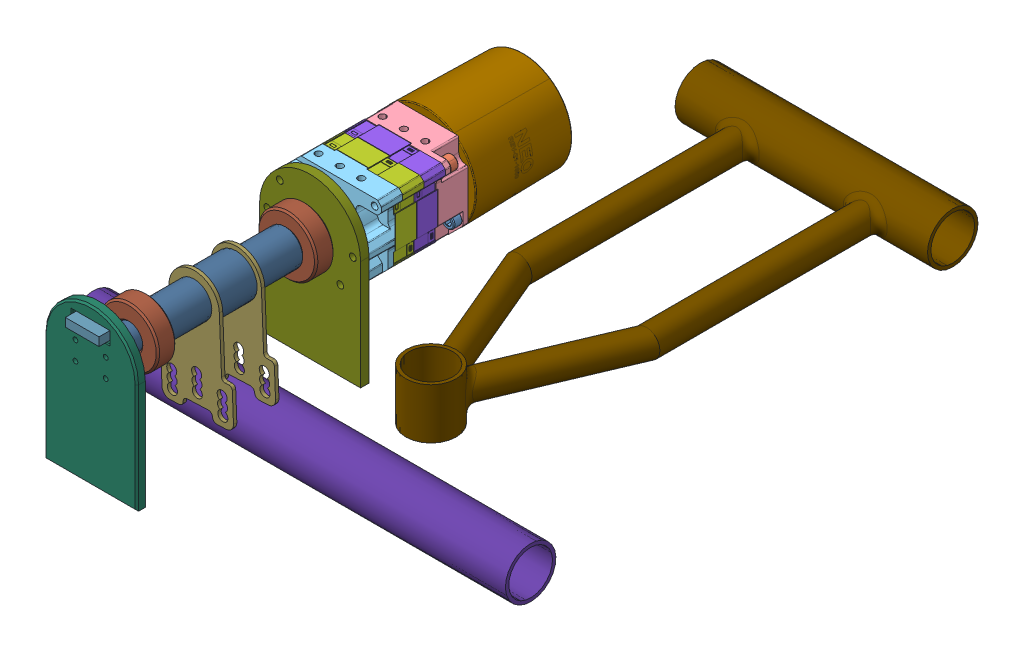
SolidWorks assembly SBW lower asm, configuration Default. Lengths in mm.
Overall size (260 177.93 457.25).
26 component instances, 18 part files, 28 mates.
Components (placement in the parent):
- MAXPlanetary 2-Stage-1: MAXPlanetary 2-Stage [Default] at origin size (89.61 89.51 122.08)
  - MAXPlanetary 2-Stage.STEP-1: MAXPlanetary 2-Stage.STEP [Default] at origin size (89.61 89.51 122.08)
    - REV-25-2109_2-Stage (No Shaft, For NEO).STEP-1: REV-25-2109_2-Stage (No Shaft, For NEO).STEP [Default] at origin size (65.15 54.03 73.34)
      - REV-25-2107_2-Stage.STEP-1: REV-25-2107_2-Stage.STEP [Default] at (0 0 6.35) x (-1 0 0) z (0 0 -1) size (65.15 54.03 73.34)
        - #10 Socket Head Cap Screws_0.500in Long.STEP-1: #10 Socket Head Cap Screws_0.500in Long.STEP [Default] at (21.1355 14.0872 12.7) x (0.923728 0.383049 0) z (0.383049 -0.923728 0) size (7.94 17.53 7.94)
        - #10 Socket Head Cap Screws_0.500in Long.STEP-2: #10 Socket Head Cap Screws_0.500in Long.STEP [Default] at (-21.1355 -14.0872 12.7) x (0.923728 0.383049 0) z (0.383049 -0.923728 0) size (7.94 17.53 7.94)
        - #10 Socket Head Cap Screws_1.500in Long.STEP-1: #10 Socket Head Cap Screws_1.500in Long.STEP [Default] at (-26.9919 21.4312 0) x (0.777574 0.628792 0) z (-0.628792 0.777574 0) size (7.94 42.93 7.94)
        - #10 Socket Head Cap Screws_1.500in Long.STEP-2: #10 Socket Head Cap Screws_1.500in Long.STEP [Default] at (26.9919 -21.4312 0) x (0.777574 0.628792 0) z (-0.628792 0.777574 0) size (7.94 42.93 7.94)
        - #10-32 Button Head Cap Screws_0.500in Long.STEP-1: #10-32 Button Head Cap Screws_0.500in Long.STEP [Default] at (0 0 -35.2425) x (0.655967 -0.754789 0) z (-0.754789 -0.655967 0) size (9.17 15.27 9.17)
      - REV-21-2106.STEP-1: REV-21-2106.STEP [Default] at origin size (61.91 50.8 19.05)
      - REV-21-2104.STEP-1: REV-21-2104.STEP [Default] at (0 0 44.45) x (0 0 1) z (-1 0 0) size (23.2 50.8 61.92)
      - REV-21-2108.STEP-1: REV-21-2108.STEP [Default] at (0 0 7.0985) x (-0.554615 -0.832107 0) z (0 0 -1) size (25.4 25.4 14.94)
    - REV-21-2101.STEP-1: REV-21-2101.STEP [Default] at (0 0 28.575) size (61.91 50.8 16.85)
    - REV-21-2102.STEP-1: REV-21-2102.STEP [Default] at (0 0 15.875) size (61.91 50.8 16.85)
    - REV-21-1650.STEP-1: REV-21-1650.STEP [Default] at (0 0 -9.525) x (0.554615 0.832107 0) z (0 0 1) size (64.41 64.76 93.26)
- shaft-1: shaft [Default] at (0 0 42.8625) x (0 0 1) z (-0.999764 0.021721 0) size (138 25 25)
- deep groove bearing 6202-1: deep groove bearing 6202 [默认] at (0 0 61.8625) size (35 35 11)
- shaft link-1: shaft link [默认] at (0 0 100.8625) x (0.999188 0.040288 0) z (0 0 1) size (42.5 73 2)
- shaft link-2: shaft link [默认] at (0 0 125.8625) x (0.999188 0.040288 0) z (0 0 1) size (42.5 73 2)
- AS5047P magnet-1: AS5047P magnet [Default] at (0 0 180.8625) x (1 0 0) z (0 1 0) size (6 2.5 6)
- deep groove bearing 6202-2: deep groove bearing 6202 [默认] at (0 0 155.8625) size (35 35 11)
- AS5047P-1: AS5047P [Default] at (0 6.4979 182.3625) size (22 28 12)
- lower AS5047P mount-1: lower AS5047P mount [Default] at (0 0 189.3625) x (0 0 -1) z (1 0 0) size (5 92.5 55)
- BLDC mount 1-1: BLDC mount 1 [默认] at (0 0 53.975) size (60 95 5)
- middle frame-1: middle frame [默认] at (-130 -110.5456 57.9191) x (0 -0.537919 0.842996) z (1 0 0) size (30 30 260)
- sw frame-1: sw frame [默认] at (0 -118.6918 -232.8837) x (0 0 -1) z (0 1 0) size (265 150 30)
Mates (geometry in assembly coordinates):
- front: coincident aligned: plane of MAXPlanetary 2-Stage-1 through (0 0 0) normal (0 0 1)
- top: coincident aligned: plane of MAXPlanetary 2-Stage-1 through (0 0 0) normal (0 1 0)
- right: coincident aligned: plane of MAXPlanetary 2-Stage-1 through (0 0 0) normal (1 0 0)
- 重合2: coincident anti-aligned: plane of MAXPlanetary 2-Stage-1/MAXPlanetary 2-Stage.STEP-1/REV-25-2109_2-Stage (No Shaft, For NEO).STEP-1/REV-21-2104.STEP-1 through (0 0 42.8625) normal (0 0 1); plane of shaft-1 through (0 0 42.8625) normal (0 0 -1)
- 同心1: concentric anti-aligned: circle of MAXPlanetary 2-Stage-1/MAXPlanetary 2-Stage.STEP-1/REV-25-2109_2-Stage (No Shaft, For NEO).STEP-1/REV-21-2104.STEP-1; cylinder of shaft-1 through (0 0 72.8625) axis (0 0 -1) radius 7.5
- 平行1: parallel anti-aligned: plane of MAXPlanetary 2-Stage-1/MAXPlanetary 2-Stage.STEP-1/REV-25-2109_2-Stage (No Shaft, For NEO).STEP-1/REV-21-2104.STEP-1 through (0.1594 7.3379 42.8625) normal (0.481071 -0.876682 0); plane of shaft-1 through (0.1593 7.3306 57.8625) normal (-0.481071 0.876682 0)
- 同心2: concentric aligned: cylinder of shaft-1 through (0 0 72.8625) axis (0 0 -1) radius 7.5; cylinder of deep groove bearing 6202-1 through (0 0 72.8625) axis (0 0 -1) radius 7.5
- 重合3: coincident anti-aligned: plane of shaft-1 through (0 0 72.8625) normal (0 0 -1); plane of deep groove bearing 6202-1 through (0 0 72.8625) normal (0 0 1)
- 同心3: concentric aligned: cylinder of shaft-1 through (0 0 102.8625) axis (0 0 -1) radius 10.5; cylinder of shaft link-1 through (0 0 102.8625) axis (0 0 -1) radius 10.5
- 重合4: coincident anti-aligned: plane of shaft-1 through (0 0 102.8625) normal (0 0 -1); plane of shaft link-1 through (-9.0049 -55.9082 102.8625) normal (0 0 1)
- 同心4: concentric aligned: cylinder of shaft-1 through (0 0 155.8625) axis (0 0 -1) radius 10.5; cylinder of shaft link-2 through (0 0 127.8625) axis (0 0 -1) radius 10.5
- 重合5: coincident anti-aligned: plane of shaft-1 through (0 0 125.8625) normal (0 0 1); plane of shaft link-2 through (-9.0049 -55.9082 125.8625) normal (0 0 -1)
- 重合6: coincident aligned: plane of shaft link-1 through (-14.9878 -0.6043 102.8625) normal (-0.999188 -0.040288 0); plane of shaft link-2 through (-14.9878 -0.6043 127.8625) normal (-0.999188 -0.040288 0)
- 重合7: coincident anti-aligned: plane of shaft-1 through (0 0 178.3625) normal (0 0 1); plane of AS5047P magnet-1 through (0 0 178.3625) normal (0 0 -1)
- 同心5: concentric aligned: cylinder of shaft-1 through (0 0 178.3625) axis (0 0 1) radius 3.5; cylinder of AS5047P magnet-1 through (0 0 178.3625) axis (0 0 1) radius 3
- 同心6: concentric aligned: cylinder of shaft-1 through (0 0 180.8625) axis (0 0 -1) radius 7.5; cylinder of deep groove bearing 6202-2 through (0 0 166.8625) axis (0 0 -1) radius 7.5
- 重合8: coincident anti-aligned: plane of shaft-1 through (0 0 155.8625) normal (0 0 1); plane of deep groove bearing 6202-2 through (0 0 155.8625) normal (0 0 -1)
- 距离1: distance = 1.5 mm anti-aligned: plane of AS5047P-1 through (0 6.4979 182.3625) normal (0 0 -1); plane of AS5047P magnet-1 through (0 0 180.8625) normal (0 0 1)
- 同心7: concentric: cylinder of AS5047P magnet-1 through (0 0 178.3625) axis (0 0 1) radius 3; point of AS5047P-1
- 平行4: parallel aligned: plane of MAXPlanetary 2-Stage-1/MAXPlanetary 2-Stage.STEP-1/REV-25-2109_2-Stage (No Shaft, For NEO).STEP-1/REV-21-2104.STEP-1 through (-30.1625 0 23.2597) normal (-1 0 0); plane of AS5047P-1 through (-11 20.4979 184.3625) normal (-1 0 0)
- 重合15: coincident anti-aligned: plane of AS5047P-1 through (0 6.4979 184.3625) normal (0 0 1); plane of lower AS5047P mount-1 through (0 0 184.3625) normal (0 0 -1)
- 同心8: concentric aligned: cylinder of AS5047P-1 through (-9 5.5 184.3625) axis (0 0 -1) radius 1.3; cylinder of lower AS5047P mount-1 through (-9 5.5 189.3625) axis (0 0 -1) radius 1.4
- 同心9: concentric aligned: cylinder of AS5047P-1 through (9 -5.5 184.3625) axis (0 0 -1) radius 1.3; cylinder of lower AS5047P mount-1 through (9 -5.5 189.3625) axis (0 0 -1) radius 1.4
- 同心10: concentric aligned: cylinder of shaft-1 through (0 0 72.8625) axis (0 0 -1) radius 7.5; cylinder of BLDC mount 1-1 through (0 0 58.975) axis (0 0 -1) radius 12.5
- 同心11: concentric anti-aligned: cylinder of MAXPlanetary 2-Stage-1/MAXPlanetary 2-Stage.STEP-1/REV-25-2109_2-Stage (No Shaft, For NEO).STEP-1/REV-21-2104.STEP-1 through (-17.9605 17.9605 53.975) axis (0 0 1) radius 2.0193; cylinder of BLDC mount 1-1 through (-17.96 17.96 58.975) axis (0 0 -1) radius 2
- 重合16: coincident anti-aligned: plane of MAXPlanetary 2-Stage-1/MAXPlanetary 2-Stage.STEP-1/REV-25-2109_2-Stage (No Shaft, For NEO).STEP-1/REV-21-2104.STEP-1 through (0 0 53.975) normal (0 0 1); plane of BLDC mount 1-1 through (0 0 53.975) normal (0 0 -1)
- 距离2: distance = 130 mm: plane of assembly through (0 0 0) normal (1 0 0); plane of assembly; plane of middle frame-1 through (130 -110.5456 57.9191) normal (1 0 0)
- 距离8: distance = 55 mm aligned: plane of sw frame-1 through (-75 -118.6918 -247.8837) normal (-1 0 0); plane of middle frame-1 through (-130 -110.5456 57.9191) normal (-1 0 0)
